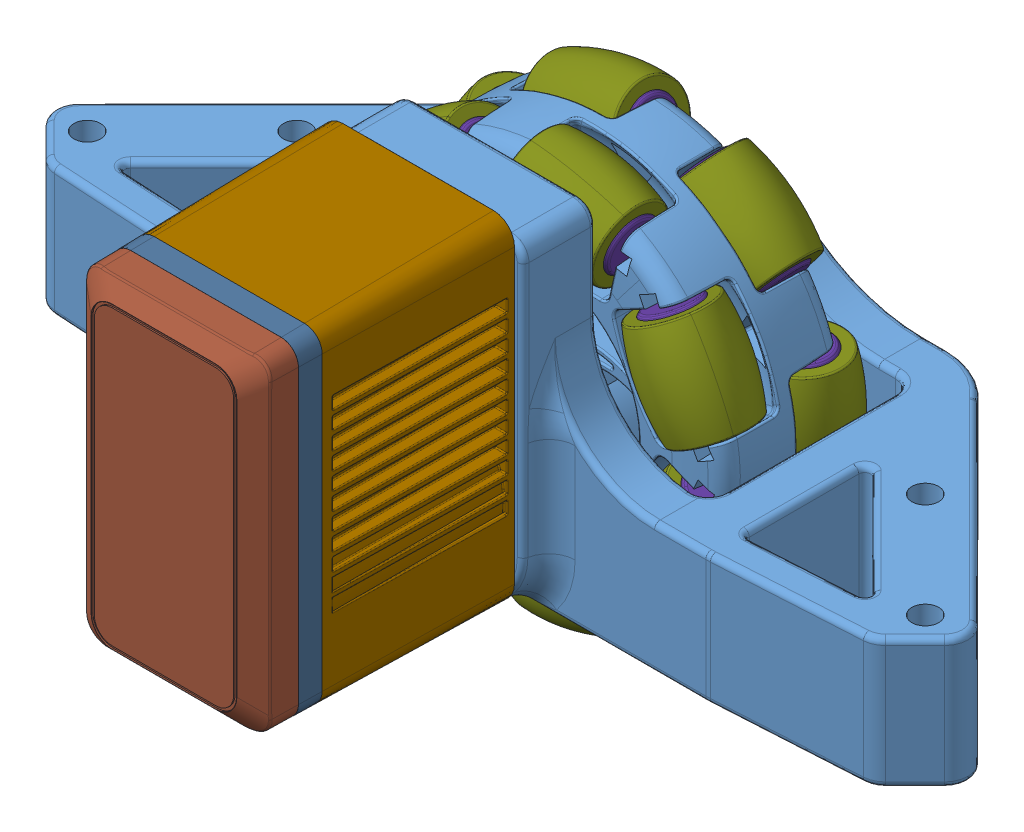
SolidWorks assembly holo_bracket_v1_testfit, configuration Default. Lengths in mm.
Overall size (156.42 97.03 100.21).
88 component instances, 22 part files, 13 mates.
Components (placement in the parent):
- holo_bracket_v2-1: holo_bracket_v2 [Default] at (-4.6322 -25.0688 0.2151) size (156.42 56.7 55.6)
- V5 Smart Motor (276-4840) no cap-1: V5 Smart Motor (276-4840) no cap [Default] at (-4.6322 6.6812 47.4651) x (0 -1 0) z (0 0 -1) size (59.01 35.33 59.91)
  - V5 Smart Motor (276-4840).step-1: V5 Smart Motor (276-4840).step [Default] at origin size (59.01 35.33 59.91)
    - 276-4840-900 Rev6_Instruction.step-1: 276-4840-900 Rev6_Instruction.step [Default] at (-14.3 0 -17.2) size (52.79 15.94 38.15)
      - 276-4840-901 Rev6.step-1: 276-4840-901 Rev6.step [Default] at (10.75 -10.05 17.8) x (-1 0 0) z (0 0 1) size (49.9 1.6 38.15)
      - 276-4840-902 Rev2.step-1: 276-4840-902 Rev2.step [Default] at (31.25 -9.25 6.2) x (0 0 -1) z (0 -1 0) size (10.35 11.39 15.94)
      - 276-4840-022 Rev4.step-1: 276-4840-022 Rev4.step [Default] at (31.25 -9.25 6.2) x (0 0 -1) z (1 0 0) size (10.26 9.1 5.51)
    - 276-4840-110 Rev10_Instruction.step-1: 276-4840-110 Rev10_Instruction.step [Default] at (12.7 0 14.7) size (35.33 35.33 31.1)
      - 276-4840-061 Rev7_Ring_Gear_Fixed01 .6 Rev3.step-1: 276-4840-061 Rev7_Ring_Gear_Fixed01 .6 Rev3.step [Default] at origin size (28.79 28.39 24.6)
      - 276-4840-018 Rev6.step-1: 276-4840-018 Rev6.step [Default] at (0 0 6.7) x (-0.483174 0.875524 0) z (0 0 1) size (26 26 12.3)
      - 276-4840-059 Rev2.step-1: 276-4840-059 Rev2.step [Default] at (0 0 10.3) size (28.4 28.4 8.5)
      - 276-4840-062 Rev1.step-1: 276-4840-062 Rev1.step [Default] at (-12.1353 8.8168 12.3) x (0.956835 -0.290632 0) z (-0.290632 -0.956835 0) size (3.2 6.56 3.2)
      - 276-4840-062 Rev1.step-2: 276-4840-062 Rev1.step [Default] at (12.1353 8.8168 12.3) x (0.978427 0.206591 0) z (0.206591 -0.978427 0) size (3.2 6.56 3.2)
      - 276-4840-062 Rev1.step-3: 276-4840-062 Rev1.step [Default] at (-12.1353 -8.8168 12.3) x (0.72563 0.688086 0) z (0.688086 -0.72563 0) size (3.2 6.56 3.2)
    - 276-4840-001 Rev38.step-1: 276-4840-001 Rev38.step [Default] at origin size (57.3 33 46.9)
    - 276-4840-005 Rev27.step-1: 276-4840-005 Rev27.step [Default] at (0 0 -17.95) size (56.17 31.87 12.9)
    - 276-4840-004 Rev16.step-1: 276-4840-004 Rev16.step [Default] at (0 0 -19.2) size (56.01 31.71 9.21)
    - 276-4840-009 Rev3.step-1: 276-4840-009 Rev3.step [Default] at (25.45 13.5 15.7) x (0.19987 -0.979823 0) z (-0.979823 -0.19987 0) size (3.4 41.31 4.34)
    - 276-4840-009 Rev3.step-2: 276-4840-009 Rev3.step [Default] at (-25.45 -13.5 15.7) x (-0.998855 0.047836 0) z (0.047836 0.998855 0) size (3.4 41.31 4.34)
    - 276-4840-009 Rev3.step-3: 276-4840-009 Rev3.step [Default] at (25.45 -13.5 15.7) x (-0.975374 0.220559 0) z (0.220559 0.975374 0) size (3.4 41.31 4.34)
    - 276-4840-009 Rev3.step-4: 276-4840-009 Rev3.step [Default] at (-25.45 13.5 15.7) x (-0.922256 0.38658 0) z (0.38658 0.922256 0) size (3.4 41.31 4.34)
    - 276-4840-025 Rev19.step-1: 276-4840-025 Rev19.step [Default] at (12.7 0 -22.63) x (-0.993315 0.115437 0) z (0 0 1) size (14.82 14.83 35.18)
- 0.375_ ID x 0.875_ OD x 0.281_ WD (Radial Bearing) (217-3239)-1: 0.375_ ID x 0.875_ OD x 0.281_ WD (Radial Bearing) (217-3239) [Default] at (-4.6322 -6.0188 -24.4723) x (0 0 1) z (-1 0 0) size (7.14 22.23 22.23)
- 0.375in_ID_Bearing_Insert-1: 0.375in_ID_Bearing_Insert [Default] at (-4.6322 -6.0188 -24.4723) size (9.4 9.4 7.14)
- 2.75 Omni with inserts (276-1902) -1: 2.75 Omni with inserts (276-1902)  [Default] at (46.131 17.9191 -68.0616) x (-0.794609 0.607122 0) z (0 0 1) size (87.15 87.98 47.75)
  - 2.75 Omni-Directional Wheel - Double Roller (276-1902) -1: 2.75 Omni-Directional Wheel - Double Roller (276-1902)  [Default] at (25.8037 49.8406 68.5807) size (87.15 87.98 47.75)
    - 2.75 Omni-Directional Wheel - Double Roller (276-1902) .step-1: 2.75 Omni-Directional Wheel - Double Roller (276-1902) .step [Default] at origin size (87.15 87.98 47.75)
      - 276-1902-010 Rev1.step-1: 276-1902-010 Rev1.step [Default] at (0 27.5 8) x (1 0 0) z (0 0.828233 0.560383) size (23 27.81 20.35)
        - 276-1902-011 Rev1.step-1: 276-1902-011 Rev1.step [Default] at (0 -6.325 -26.7627) x (1 0 0) z (0 -0.973191 0.23) size (16.5 15 25.03)
        - 276-1902-012 Rev1.step-1: 276-1902-012 Rev1.step [Default] at origin size (17.5 10.34 18.34)
        - 276-1902-003 Rev1.step-1: 276-1902-003 Rev1.step [Default] x (0 -0.928523 0.371275) z (1 0 0) size (2 2 23)
      - 276-1902-010 Rev1.step-2: 276-1902-010 Rev1.step [Default] at (0 -27.5 -8) x (1 0 0) z (0 0.410464 0.911877) size (23 27.81 20.35)
        - 276-1902-011 Rev1.step-1: 276-1902-011 Rev1.step [Default] at (0 -6.325 -26.7627) x (1 0 0) z (0 -0.973191 0.23) size (16.5 15 25.03)
        - 276-1902-012 Rev1.step-1: 276-1902-012 Rev1.step [Default] at origin size (17.5 10.34 18.34)
        - 276-1902-003 Rev1.step-1: 276-1902-003 Rev1.step [Default] x (0 -0.928523 0.371275) z (1 0 0) size (2 2 23)
      - 276-1902-010 Rev1.step-3: 276-1902-010 Rev1.step [Default] at (-21.5004 -17.146 -8) x (0.62349 -0.781831 0) z (0.320913 0.25592 0.911877) size (23 27.81 20.35)
        - 276-1902-011 Rev1.step-1: 276-1902-011 Rev1.step [Default] at (0 -6.325 -26.7627) x (1 0 0) z (0 -0.973191 0.23) size (16.5 15 25.03)
        - 276-1902-012 Rev1.step-1: 276-1902-012 Rev1.step [Default] at origin size (17.5 10.34 18.34)
        - 276-1902-003 Rev1.step-1: 276-1902-003 Rev1.step [Default] x (0 -0.928523 0.371275) z (1 0 0) size (2 2 23)
      - 276-1902-010 Rev1.step-4: 276-1902-010 Rev1.step [Default] at (-26.8105 6.1193 -8) x (-0.222521 -0.974928 0) z (0.400172 -0.091337 0.911877) size (23 27.81 20.35)
        - 276-1902-011 Rev1.step-1: 276-1902-011 Rev1.step [Default] at (0 -6.325 -26.7627) x (1 0 0) z (0 -0.973191 0.23) size (16.5 15 25.03)
        - 276-1902-012 Rev1.step-1: 276-1902-012 Rev1.step [Default] at origin size (17.5 10.34 18.34)
        - 276-1902-003 Rev1.step-1: 276-1902-003 Rev1.step [Default] x (0 -0.928523 0.371275) z (1 0 0) size (2 2 23)
      - 276-1902-010 Rev1.step-5: 276-1902-010 Rev1.step [Default] at (-11.9318 24.7766 -8) x (-0.900969 -0.433884 0) z (0.178093 -0.369815 0.911877) size (23 27.81 20.35)
        - 276-1902-011 Rev1.step-1: 276-1902-011 Rev1.step [Default] at (0 -6.325 -26.7627) x (1 0 0) z (0 -0.973191 0.23) size (16.5 15 25.03)
        - 276-1902-012 Rev1.step-1: 276-1902-012 Rev1.step [Default] at origin size (17.5 10.34 18.34)
        - 276-1902-003 Rev1.step-1: 276-1902-003 Rev1.step [Default] x (0 -0.928523 0.371275) z (1 0 0) size (2 2 23)
      - 276-1902-010 Rev1.step-6: 276-1902-010 Rev1.step [Default] at (11.9318 24.7766 -8) x (-0.900969 0.433884 0) z (-0.178093 -0.369815 0.911877) size (23 27.81 20.35)
        - 276-1902-011 Rev1.step-1: 276-1902-011 Rev1.step [Default] at (0 -6.325 -26.7627) x (1 0 0) z (0 -0.973191 0.23) size (16.5 15 25.03)
        - 276-1902-012 Rev1.step-1: 276-1902-012 Rev1.step [Default] at origin size (17.5 10.34 18.34)
        - 276-1902-003 Rev1.step-1: 276-1902-003 Rev1.step [Default] x (0 -0.928523 0.371275) z (1 0 0) size (2 2 23)
      - 276-1902-010 Rev1.step-7: 276-1902-010 Rev1.step [Default] at (26.8105 6.1193 -8) x (-0.222521 0.974928 0) z (-0.400172 -0.091337 0.911877) size (23 27.81 20.35)
        - 276-1902-011 Rev1.step-1: 276-1902-011 Rev1.step [Default] at (0 -6.325 -26.7627) x (1 0 0) z (0 -0.973191 0.23) size (16.5 15 25.03)
        - 276-1902-012 Rev1.step-1: 276-1902-012 Rev1.step [Default] at origin size (17.5 10.34 18.34)
        - 276-1902-003 Rev1.step-1: 276-1902-003 Rev1.step [Default] x (0 -0.928523 0.371275) z (1 0 0) size (2 2 23)
      - 276-1902-010 Rev1.step-8: 276-1902-010 Rev1.step [Default] at (21.5004 -17.146 -8) x (0.62349 0.781831 0) z (-0.320913 0.25592 0.911877) size (23 27.81 20.35)
        - 276-1902-011 Rev1.step-1: 276-1902-011 Rev1.step [Default] at (0 -6.325 -26.7627) x (1 0 0) z (0 -0.973191 0.23) size (16.5 15 25.03)
        - 276-1902-012 Rev1.step-1: 276-1902-012 Rev1.step [Default] at origin size (17.5 10.34 18.34)
        - 276-1902-003 Rev1.step-1: 276-1902-003 Rev1.step [Default] x (0 -0.928523 0.371275) z (1 0 0) size (2 2 23)
      - 276-1902-010 Rev1.step-9: 276-1902-010 Rev1.step [Default] at (21.5004 17.146 8) x (0.62349 -0.781831 0) z (0.647539 0.516395 0.560383) size (23 27.81 20.35)
        - 276-1902-011 Rev1.step-1: 276-1902-011 Rev1.step [Default] at (0 -6.325 -26.7627) x (1 0 0) z (0 -0.973191 0.23) size (16.5 15 25.03)
        - 276-1902-012 Rev1.step-1: 276-1902-012 Rev1.step [Default] at origin size (17.5 10.34 18.34)
        - 276-1902-003 Rev1.step-1: 276-1902-003 Rev1.step [Default] x (0 -0.928523 0.371275) z (1 0 0) size (2 2 23)
      - 276-1902-010 Rev1.step-10: 276-1902-010 Rev1.step [Default] at (26.8105 -6.1193 8) x (-0.222521 -0.974928 0) z (0.807468 -0.184299 0.560383) size (23 27.81 20.35)
        - 276-1902-011 Rev1.step-1: 276-1902-011 Rev1.step [Default] at (0 -6.325 -26.7627) x (1 0 0) z (0 -0.973191 0.23) size (16.5 15 25.03)
        - 276-1902-012 Rev1.step-1: 276-1902-012 Rev1.step [Default] at origin size (17.5 10.34 18.34)
        - 276-1902-003 Rev1.step-1: 276-1902-003 Rev1.step [Default] x (0 -0.928523 0.371275) z (1 0 0) size (2 2 23)
      - 276-1902-010 Rev1.step-11: 276-1902-010 Rev1.step [Default] at (11.9318 -24.7766 8) x (-0.900969 -0.433884 0) z (0.359357 -0.746212 0.560383) size (23 27.81 20.35)
        - 276-1902-011 Rev1.step-1: 276-1902-011 Rev1.step [Default] at (0 -6.325 -26.7627) x (1 0 0) z (0 -0.973191 0.23) size (16.5 15 25.03)
        - 276-1902-012 Rev1.step-1: 276-1902-012 Rev1.step [Default] at origin size (17.5 10.34 18.34)
        - 276-1902-003 Rev1.step-1: 276-1902-003 Rev1.step [Default] x (0 -0.928523 0.371275) z (1 0 0) size (2 2 23)
      - 276-1902-010 Rev1.step-12: 276-1902-010 Rev1.step [Default] at (-11.9318 -24.7766 8) x (-0.900969 0.433884 0) z (-0.359357 -0.746212 0.560383) size (23 27.81 20.35)
        - 276-1902-011 Rev1.step-1: 276-1902-011 Rev1.step [Default] at (0 -6.325 -26.7627) x (1 0 0) z (0 -0.973191 0.23) size (16.5 15 25.03)
        - 276-1902-012 Rev1.step-1: 276-1902-012 Rev1.step [Default] at origin size (17.5 10.34 18.34)
        - 276-1902-003 Rev1.step-1: 276-1902-003 Rev1.step [Default] x (0 -0.928523 0.371275) z (1 0 0) size (2 2 23)
      - 276-1902-010 Rev1.step-13: 276-1902-010 Rev1.step [Default] at (-26.8105 -6.1193 8) x (-0.222521 0.974928 0) z (-0.807468 -0.184299 0.560383) size (23 27.81 20.35)
        - 276-1902-011 Rev1.step-1: 276-1902-011 Rev1.step [Default] at (0 -6.325 -26.7627) x (1 0 0) z (0 -0.973191 0.23) size (16.5 15 25.03)
        - 276-1902-012 Rev1.step-1: 276-1902-012 Rev1.step [Default] at origin size (17.5 10.34 18.34)
        - 276-1902-003 Rev1.step-1: 276-1902-003 Rev1.step [Default] x (0 -0.928523 0.371275) z (1 0 0) size (2 2 23)
      - 276-1902-010 Rev1.step-14: 276-1902-010 Rev1.step [Default] at (-21.5004 17.146 8) x (0.62349 0.781831 0) z (-0.647539 0.516395 0.560383) size (23 27.81 20.35)
        - 276-1902-011 Rev1.step-1: 276-1902-011 Rev1.step [Default] at (0 -6.325 -26.7627) x (1 0 0) z (0 -0.973191 0.23) size (16.5 15 25.03)
        - 276-1902-012 Rev1.step-1: 276-1902-012 Rev1.step [Default] at origin size (17.5 10.34 18.34)
        - 276-1902-003 Rev1.step-1: 276-1902-003 Rev1.step [Default] x (0 -0.928523 0.371275) z (1 0 0) size (2 2 23)
      - 276-1902-002 Rev3.step-1: 276-1902-002 Rev3.step [Default] at origin size (66.55 66.02 25.07)
  - Metal Shaft Inserts (276-3881-002)-1: Metal Shaft Inserts (276-3881-002) [Default] at (25.8037 49.8406 79.8307) x (0 -1 0) z (1 0 0) size (10.03 5.08 10.03)
  - Metal Shaft Inserts (276-3881-002)-2: Metal Shaft Inserts (276-3881-002) [Default] at (25.8037 49.8406 57.3307) x (1 0 0) z (0 -1 0) size (10.03 5.08 10.03)
- Drive Shaft 2in-1: Drive Shaft 2in [Default] at (-4.6322 -6.0188 -126.7349) size (3.28 3.28 50.8)
- Shaft Collar (276-2010)-1: Shaft Collar (276-2010) [Default] at (-4.6322 -6.0188 -14.0329) x (0.96656 -0.256441 0) z (0 0 -1) size (11 11.35 6.6)
Mates (geometry in assembly coordinates):
- Coincident1: coincident anti-aligned: plane of holo_bracket_v2-1 through (-4.6322 -25.0688 30.2651) normal (0 0 1); plane of V5 Smart Motor (276-4840) no cap-1/V5 Smart Motor (276-4840).step-1/276-4840-001 Rev38.step-1 through (-17.5322 31.7312 30.2651) normal (0 0 -1)
- Concentric1: concentric anti-aligned: cylinder of holo_bracket_v2-1 through (-4.6322 -6.0188 25.7661) axis (0 0 -1) radius 6.35; circle of V5 Smart Motor (276-4840) no cap-1/V5 Smart Motor (276-4840).step-1/276-4840-110 Rev10_Instruction.step-1/276-4840-059 Rev2.step-1
- Parallel1: parallel: plane of holo_bracket_v2-1 through (-4.6322 31.6312 -20.99) normal (0 1 0); line of V5 Smart Motor (276-4840) no cap-1/V5 Smart Motor (276-4840).step-1/276-4840-001 Rev38.step-1 through (-17.5322 35.3312 31.2651) axis (1 0 0)
- Concentric2: concentric anti-aligned: cylinder of holo_bracket_v2-1 through (-4.6322 -6.0188 -24.4723) axis (0 0 1) radius 11.25; cylinder of 0.375_ ID x 0.875_ OD x 0.281_ WD (Radial Bearing) (217-3239)-1 through (-4.6322 -6.0188 -39.0092) axis (0 0 -1) radius 11.113
- Coincident3: coincident anti-aligned: plane of holo_bracket_v2-1 through (-4.6322 -6.0188 -24.4723) normal (0 0 1); plane of 0.375_ ID x 0.875_ OD x 0.281_ WD (Radial Bearing) (217-3239)-1 through (-4.6322 -15.5018 -24.4723) normal (0 0 -1)
- Concentric3: concentric aligned: cylinder of 0.375_ ID x 0.875_ OD x 0.281_ WD (Radial Bearing) (217-3239)-1 through (-4.6322 -6.0188 -39.0092) axis (0 0 -1) radius 4.763; cylinder of 0.375in_ID_Bearing_Insert-1 through (-4.6322 -6.0188 -17.3349) axis (0 0 -1) radius 4.7
- Coincident4: coincident anti-aligned: plane of holo_bracket_v2-1 through (-4.6322 -6.0188 -24.4723) normal (0 0 1); plane of 0.375in_ID_Bearing_Insert-1 through (-4.6322 -6.0188 -24.4723) normal (0 0 -1)
- Coincident5: coincident anti-aligned: plane of 2.75 Omni with inserts (276-1902) -1/Metal Shaft Inserts (276-3881-002)-2 through (-4.6322 -6.0188 -10.7309) normal (0 0 -1); plane of Shaft Collar (276-2010)-1 through (-4.6322 -6.0188 -10.7309) normal (0 0 1)
- Concentric5: concentric aligned: circle of 2.75 Omni with inserts (276-1902) -1/Metal Shaft Inserts (276-3881-002)-2; circle of Shaft Collar (276-2010)-1
- Concentric6: concentric anti-aligned: circle of holo_bracket_v1-1; circle of Drive Shaft 2in-1
- Coincident6: coincident anti-aligned: plane of V5 Smart Motor (276-4840) no cap-1/V5 Smart Motor (276-4840).step-1/276-4840-110 Rev10_Instruction.step-1/276-4840-018 Rev6.step-1 through (-4.6322 -6.0188 25.6651) normal (0 0 -1); plane of Drive Shaft 2in-1 through (-6.2197 -4.4313 25.6651) normal (0 0 1)
- Coincident7: coincident anti-aligned: plane of holo_bracket_v2-1 through (-4.6322 -2.8188 -17.3349) normal (0 0 1); plane of Shaft Collar (276-2010)-1 through (-4.6322 -6.0188 -17.3349) normal (0 0 -1)
- Concentric7: concentric anti-aligned: circle of holo_bracket_v1-1; circle of Shaft Collar (276-2010)-1
